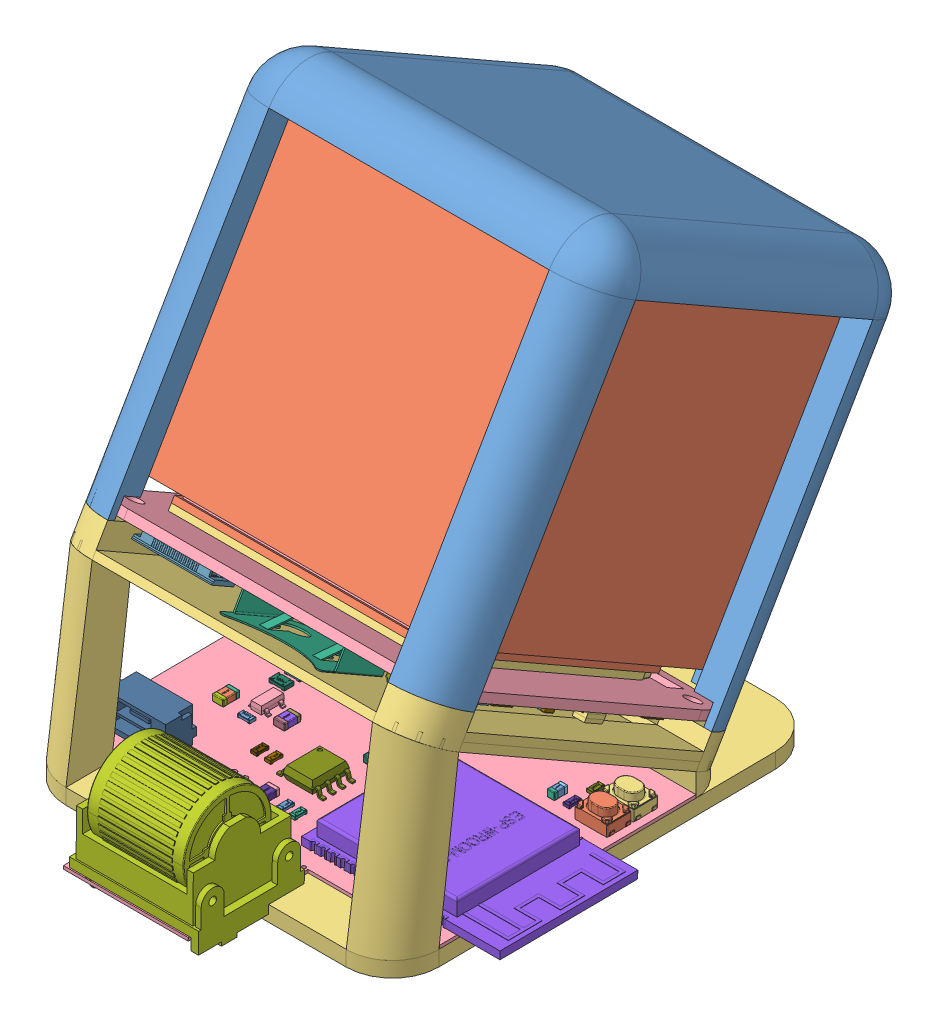
SolidWorks assembly main, configuration 默认. Lengths in mm.
Overall size (55.34 95.26 82.21).
436 component instances, 154 part files, 13 mates.
Components (placement in the parent):
- case-1: case [默认] at (0.5158 4.4817 0.3951) x (0.999924 -0.008726 -0.008727) z (0.01192 0.499915 0.865992) size (48 47.5 48)
- cubic-1: cubic [默认] at (0.3684 19.1653 -31.1742) x (0.999924 -0.008726 -0.008727) z (0.01192 0.499915 0.865992) size (40 40 40)
- stand-1: stand [默认] at (0.5158 4.4817 0.3951) x (0.01192 0.499915 0.865992) z (-0.999924 0.008726 0.008727) size (61.5 29.73 48.03)
- PCB_2020-12-27_16-28-50_2021-02-20_20-59-34-1: PCB_2020-12-27_16-28-50_2021-02-20_20-59-34 [默认] at (-66.8523 -25.1637 -60.1398) x (0.999924 -0.008726 -0.008727) z (-0.003194 -0.866031 0.499981) size (45.01 51.47 7.58)
  - PCB_2020-12-27_16-28-50_2021-02-20_20-59-34.step-1: PCB_2020-12-27_16-28-50_2021-02-20_20-59-34.step [默认] at origin size (45.01 51.47 7.58)
    - Board.step-1: Board.step [默认] at origin size (45.01 45.01 1.12)
      - Open CASCADE STEP translator 6.8 3.1.1.step-1: Open CASCADE STEP translator 6.8 3.1.1.step [默认] at (0 0 -1.1227) size (45.01 45.01 1.12)
    - C34.step-1: C34.step [默认] at origin size (2.2 1.45 0.88)
      - c0805c101k5gactu.step-1: c0805c101k5gactu.step [默认] at (159.963 120.323 -10.6426) x (1 0 0) z (0 -1 0) size (2.2 0.88 1.45)
        - Open CASCADE STEP translator 6.8 3.2.1.1.step-1: Open CASCADE STEP translator 6.8 3.2.1.1.step [默认] at origin size (2 0.86 1.43)
        - Open CASCADE STEP translator 6.8 3.2.1.2.step-1: Open CASCADE STEP translator 6.8 3.2.1.2.step [默认] at origin size (0.34 0 0.18)
        - Open CASCADE STEP translator 6.8 3.2.1.3.step-1: Open CASCADE STEP translator 6.8 3.2.1.3.step [默认] at origin size (0.41 0 0.18)
        - Open CASCADE STEP translator 6.8 3.2.1.4.step-1: Open CASCADE STEP translator 6.8 3.2.1.4.step [默认] at origin size (0.21 0 0.18)
        - Open CASCADE STEP translator 6.8 3.2.1.5.step-1: Open CASCADE STEP translator 6.8 3.2.1.5.step [默认] at origin size (0.5 0.88 1.45)
        - Open CASCADE STEP translator 6.8 3.2.1.6.step-1: Open CASCADE STEP translator 6.8 3.2.1.6.step [默认] at origin size (0.5 0.88 1.45)
    - C14.step-1: C14.step [默认] at origin size (1.45 2.2 0.88)
      - c0805c101k5gactu.step-1: c0805c101k5gactu.step [默认] at (101.7169 -30.907 -10.6426) x (0 -1 0) z (-1 0 0) size (2.2 0.88 1.45)
        - Open CASCADE STEP translator 6.8 3.2.1.1.step-1: Open CASCADE STEP translator 6.8 3.2.1.1.step [默认] at origin size (2 0.86 1.43)
        - Open CASCADE STEP translator 6.8 3.2.1.2.step-1: Open CASCADE STEP translator 6.8 3.2.1.2.step [默认] at origin size (0.34 0 0.18)
        - Open CASCADE STEP translator 6.8 3.2.1.3.step-1: Open CASCADE STEP translator 6.8 3.2.1.3.step [默认] at origin size (0.41 0 0.18)
        - Open CASCADE STEP translator 6.8 3.2.1.4.step-1: Open CASCADE STEP translator 6.8 3.2.1.4.step [默认] at origin size (0.21 0 0.18)
        - Open CASCADE STEP translator 6.8 3.2.1.5.step-1: Open CASCADE STEP translator 6.8 3.2.1.5.step [默认] at origin size (0.5 0.88 1.45)
        - Open CASCADE STEP translator 6.8 3.2.1.6.step-1: Open CASCADE STEP translator 6.8 3.2.1.6.step [默认] at origin size (0.5 0.88 1.45)
    - C13.step-1: C13.step [默认] at origin size (0.95 1.77 0.95)
      - c0603x104k3ractu.step-1: c0603x104k3ractu.step [默认] at (16.3625 164.212 -10.6426) x (0 1 0) z (1 0 0) size (1.77 0.95 0.95)
        - Open CASCADE STEP translator 6.8 3.4.1.1.step-1: Open CASCADE STEP translator 6.8 3.4.1.1.step [默认] at origin size (1.57 0.93 0.93)
        - Open CASCADE STEP translator 6.8 3.4.1.2.step-1: Open CASCADE STEP translator 6.8 3.4.1.2.step [默认] at origin size (0.24 0 0.13)
        - Open CASCADE STEP translator 6.8 3.4.1.3.step-1: Open CASCADE STEP translator 6.8 3.4.1.3.step [默认] at origin size (0.29 0 0.13)
        - Open CASCADE STEP translator 6.8 3.4.1.4.step-1: Open CASCADE STEP translator 6.8 3.4.1.4.step [默认] at origin size (0.15 0 0.13)
        - Open CASCADE STEP translator 6.8 3.4.1.5.step-1: Open CASCADE STEP translator 6.8 3.4.1.5.step [默认] at origin size (0.45 0.95 0.95)
        - Open CASCADE STEP translator 6.8 3.4.1.6.step-1: Open CASCADE STEP translator 6.8 3.4.1.6.step [默认] at origin size (0.45 0.95 0.95)
    - C12.step-1: C12.step [默认] at origin size (0.95 1.77 0.95)
      - c0603x104k3ractu.step-1: c0603x104k3ractu.step [默认] at (9.3976 164.422 -10.6426) x (0 1 0) z (1 0 0) size (1.77 0.95 0.95)
        - Open CASCADE STEP translator 6.8 3.4.1.1.step-1: Open CASCADE STEP translator 6.8 3.4.1.1.step [默认] at origin size (1.57 0.93 0.93)
        - Open CASCADE STEP translator 6.8 3.4.1.2.step-1: Open CASCADE STEP translator 6.8 3.4.1.2.step [默认] at origin size (0.24 0 0.13)
        - Open CASCADE STEP translator 6.8 3.4.1.3.step-1: Open CASCADE STEP translator 6.8 3.4.1.3.step [默认] at origin size (0.29 0 0.13)
        - Open CASCADE STEP translator 6.8 3.4.1.4.step-1: Open CASCADE STEP translator 6.8 3.4.1.4.step [默认] at origin size (0.15 0 0.13)
        - Open CASCADE STEP translator 6.8 3.4.1.5.step-1: Open CASCADE STEP translator 6.8 3.4.1.5.step [默认] at origin size (0.45 0.95 0.95)
        - Open CASCADE STEP translator 6.8 3.4.1.6.step-1: Open CASCADE STEP translator 6.8 3.4.1.6.step [默认] at origin size (0.45 0.95 0.95)
    - USB2.step-1: USB2.step [默认] at origin size (5 7.8 2.7)
      - User_Library-micro_usb_SMD_RGB8421504.step-1: User_Library-micro_usb_SMD_RGB8421504.step [默认] at (44.3599 67.8551 1.27) x (0 -1 0) z (-1 0 0) size (7.8 2.7 5)
    - R7.step-1: R7.step [默认] at origin size (1.6 0.8 0.42)
      - User_Library-Res-0603.step-1: User_Library-Res-0603.step [默认] at (87.122 80.8989 0) x (-1 0 0) z (0 1 0) size (1.6 0.42 0.8)
    - L2.step-1: L2.step [默认] at origin size (0.86 1.6 0.51)
      - CircuitWorks-RESISTOR_0603.step-1: CircuitWorks-RESISTOR_0603.step [默认] at (61.595 79.7559 0) x (0 -1 0) z (-1 0 0) size (1.6 0.51 0.86)
    - P2.step-1: P2.step [默认] at origin size (20.43 5.11 2.05)
      - 3-1734839-0_RGB8421504.step-1: 3-1734839-0_RGB8421504.step [默认] at (66.548 57.4041 1.0414) x (1 0 0) z (0 -1 0) size (20.43 2.05 5.11)
    - D4.step-1: D4.step [默认] at origin size (3.7 1.6 1.27)
      - CircuitWorks-SOD123.step-1: CircuitWorks-SOD123.step [默认] at (72.4968 69.5129 0.0508) x (1 0 0) z (0 -1 0) size (3.7 1.27 1.6)
    - D5.step-1: D5.step [默认] at origin size (1.6 3.7 1.27)
      - CircuitWorks-SOD123.step-1: CircuitWorks-SOD123.step [默认] at (87.6301 64.8969 0.0508) x (0 1 0) z (1 0 0) size (3.7 1.27 1.6)
    - C21.step-1: C21.step [默认] at origin size (1.45 2.2 0.88)
      - c0805c101k5gactu.step-1: c0805c101k5gactu.step [默认] at (98.5419 -33.828 -10.6426) x (0 -1 0) z (-1 0 0) size (2.2 0.88 1.45)
        - Open CASCADE STEP translator 6.8 3.2.1.1.step-1: Open CASCADE STEP translator 6.8 3.2.1.1.step [默认] at origin size (2 0.86 1.43)
        - Open CASCADE STEP translator 6.8 3.2.1.2.step-1: Open CASCADE STEP translator 6.8 3.2.1.2.step [默认] at origin size (0.34 0 0.18)
        - Open CASCADE STEP translator 6.8 3.2.1.3.step-1: Open CASCADE STEP translator 6.8 3.2.1.3.step [默认] at origin size (0.41 0 0.18)
        - Open CASCADE STEP translator 6.8 3.2.1.4.step-1: Open CASCADE STEP translator 6.8 3.2.1.4.step [默认] at origin size (0.21 0 0.18)
        - Open CASCADE STEP translator 6.8 3.2.1.5.step-1: Open CASCADE STEP translator 6.8 3.2.1.5.step [默认] at origin size (0.5 0.88 1.45)
        - Open CASCADE STEP translator 6.8 3.2.1.6.step-1: Open CASCADE STEP translator 6.8 3.2.1.6.step [默认] at origin size (0.5 0.88 1.45)
    - C24.step-1: C24.step [默认] at origin size (1.45 2.2 0.88)
      - c0805c101k5gactu.step-1: c0805c101k5gactu.step [默认] at (2.51 156.471 -10.6426) x (0 1 0) z (1 0 0) size (2.2 0.88 1.45)
        - Open CASCADE STEP translator 6.8 3.2.1.1.step-1: Open CASCADE STEP translator 6.8 3.2.1.1.step [默认] at origin size (2 0.86 1.43)
        - Open CASCADE STEP translator 6.8 3.2.1.2.step-1: Open CASCADE STEP translator 6.8 3.2.1.2.step [默认] at origin size (0.34 0 0.18)
        - Open CASCADE STEP translator 6.8 3.2.1.3.step-1: Open CASCADE STEP translator 6.8 3.2.1.3.step [默认] at origin size (0.41 0 0.18)
        - Open CASCADE STEP translator 6.8 3.2.1.4.step-1: Open CASCADE STEP translator 6.8 3.2.1.4.step [默认] at origin size (0.21 0 0.18)
        - Open CASCADE STEP translator 6.8 3.2.1.5.step-1: Open CASCADE STEP translator 6.8 3.2.1.5.step [默认] at origin size (0.5 0.88 1.45)
        - Open CASCADE STEP translator 6.8 3.2.1.6.step-1: Open CASCADE STEP translator 6.8 3.2.1.6.step [默认] at origin size (0.5 0.88 1.45)
    - U7.step-1: U7.step [默认] at origin size (2.5 3 1.1)
      - CircuitWorks-SOT-23-5.step-1: CircuitWorks-SOT-23-5.step [默认] at (84.308 68.2431 -0.5131) x (0 1 0) z (1 0 0) size (3 1.1 2.5)
    - U5.step-1: U5.step [默认] at origin size (7 7 0.55)
      - User_Library-UFQFPN48.step-1: User_Library-UFQFPN48.step [默认] at (57.0029 73.1959 0) x (-1 0 0) z (0 0 1) size (7 7 0.55)
    - R13.step-1: R13.step [默认] at origin size (0.8 1.6 0.42)
      - User_Library-Res-0603.step-1: User_Library-Res-0603.step [默认] at (78.3388 65.957 0) x (0 1 0) z (1 0 0) size (1.6 0.42 0.8)
    - U4.step-1: U4.step [默认] at origin size (19.57 12.72 3.54)
      - User_Library-BK-885-TR.step-1: User_Library-BK-885-TR.step [默认] at (69.4691 84.328 0) x (1 0 0) z (0 -1 0) size (19.57 3.54 12.72)
    - U3.step-1: U3.step [默认] at origin size (0.8 1.6 0.42)
      - User_Library-Res-0603.step-1: User_Library-Res-0603.step [默认] at (61.3211 52.876 0) x (0 -1 0) z (-1 0 0) size (1.6 0.42 0.8)
    - C27.step-1: C27.step [默认] at origin size (0.95 1.77 0.95)
      - c0603x104k3ractu.step-1: c0603x104k3ractu.step [默认] at (123.9324 -30.647 -10.6426) x (0 -1 0) z (-1 0 0) size (1.77 0.95 0.95)
        - Open CASCADE STEP translator 6.8 3.4.1.1.step-1: Open CASCADE STEP translator 6.8 3.4.1.1.step [默认] at origin size (1.57 0.93 0.93)
        - Open CASCADE STEP translator 6.8 3.4.1.2.step-1: Open CASCADE STEP translator 6.8 3.4.1.2.step [默认] at origin size (0.24 0 0.13)
        - Open CASCADE STEP translator 6.8 3.4.1.3.step-1: Open CASCADE STEP translator 6.8 3.4.1.3.step [默认] at origin size (0.29 0 0.13)
        - Open CASCADE STEP translator 6.8 3.4.1.4.step-1: Open CASCADE STEP translator 6.8 3.4.1.4.step [默认] at origin size (0.15 0 0.13)
        - Open CASCADE STEP translator 6.8 3.4.1.5.step-1: Open CASCADE STEP translator 6.8 3.4.1.5.step [默认] at origin size (0.45 0.95 0.95)
        - Open CASCADE STEP translator 6.8 3.4.1.6.step-1: Open CASCADE STEP translator 6.8 3.4.1.6.step [默认] at origin size (0.45 0.95 0.95)
    - C20.step-1: C20.step [默认] at origin size (3.7 1.95 1.8)
      - c1206x223j2gacauto.step-1: c1206x223j2gacauto.step [默认] at (174.9253 96.5054 -10.6426) x (1 0 0) z (0 -1 0) size (3.7 1.8 1.95)
        - Open CASCADE STEP translator 6.8 3.20.1.1.step-1: Open CASCADE STEP translator 6.8 3.20.1.1.step [默认] at origin size (3.5 1.78 1.93)
        - Open CASCADE STEP translator 6.8 3.20.1.2.step-1: Open CASCADE STEP translator 6.8 3.20.1.2.step [默认] at origin size (0.7 0 0.37)
        - Open CASCADE STEP translator 6.8 3.20.1.3.step-1: Open CASCADE STEP translator 6.8 3.20.1.3.step [默认] at origin size (0.85 0 0.37)
        - Open CASCADE STEP translator 6.8 3.20.1.4.step-1: Open CASCADE STEP translator 6.8 3.20.1.4.step [默认] at origin size (0.44 0 0.37)
        - Open CASCADE STEP translator 6.8 3.20.1.5.step-1: Open CASCADE STEP translator 6.8 3.20.1.5.step [默认] at origin size (0.6 1.8 1.95)
        - Open CASCADE STEP translator 6.8 3.20.1.6.step-1: Open CASCADE STEP translator 6.8 3.20.1.6.step [默认] at origin size (0.6 1.8 1.95)
    - X3.step-1: X3.step [默认] at origin size (1.5 3.2 0.91)
      - crystal_rtf3215.step-1: crystal_rtf3215.step [默认] at (66.167 69.4691 0) x (0 1 0) z (1 0 0) size (3.2 0.91 1.5)
    - C28.step-1: C28.step [默认] at origin size (1.45 2.2 0.88)
      - c0805c101k5gactu.step-1: c0805c101k5gactu.step [默认] at (25.644 150.077 -10.6426) x (0 1 0) z (1 0 0) size (2.2 0.88 1.45)
        - Open CASCADE STEP translator 6.8 3.2.1.1.step-1: Open CASCADE STEP translator 6.8 3.2.1.1.step [默认] at origin size (2 0.86 1.43)
        - Open CASCADE STEP translator 6.8 3.2.1.2.step-1: Open CASCADE STEP translator 6.8 3.2.1.2.step [默认] at origin size (0.34 0 0.18)
        - Open CASCADE STEP translator 6.8 3.2.1.3.step-1: Open CASCADE STEP translator 6.8 3.2.1.3.step [默认] at origin size (0.41 0 0.18)
        - Open CASCADE STEP translator 6.8 3.2.1.4.step-1: Open CASCADE STEP translator 6.8 3.2.1.4.step [默认] at origin size (0.21 0 0.18)
        - Open CASCADE STEP translator 6.8 3.2.1.5.step-1: Open CASCADE STEP translator 6.8 3.2.1.5.step [默认] at origin size (0.5 0.88 1.45)
        - Open CASCADE STEP translator 6.8 3.2.1.6.step-1: Open CASCADE STEP translator 6.8 3.2.1.6.step [默认] at origin size (0.5 0.88 1.45)
    - C29.step-1: C29.step [默认] at origin size (1.45 2.2 0.88)
      - c0805c101k5gactu.step-1: c0805c101k5gactu.step [默认] at (102.7329 -43.6071 -10.6426) x (0 -1 0) z (-1 0 0) size (2.2 0.88 1.45)
        - Open CASCADE STEP translator 6.8 3.2.1.1.step-1: Open CASCADE STEP translator 6.8 3.2.1.1.step [默认] at origin size (2 0.86 1.43)
        - Open CASCADE STEP translator 6.8 3.2.1.2.step-1: Open CASCADE STEP translator 6.8 3.2.1.2.step [默认] at origin size (0.34 0 0.18)
        - Open CASCADE STEP translator 6.8 3.2.1.3.step-1: Open CASCADE STEP translator 6.8 3.2.1.3.step [默认] at origin size (0.41 0 0.18)
        - Open CASCADE STEP translator 6.8 3.2.1.4.step-1: Open CASCADE STEP translator 6.8 3.2.1.4.step [默认] at origin size (0.21 0 0.18)
        - Open CASCADE STEP translator 6.8 3.2.1.5.step-1: Open CASCADE STEP translator 6.8 3.2.1.5.step [默认] at origin size (0.5 0.88 1.45)
        - Open CASCADE STEP translator 6.8 3.2.1.6.step-1: Open CASCADE STEP translator 6.8 3.2.1.6.step [默认] at origin size (0.5 0.88 1.45)
    - C30.step-1: C30.step [默认] at origin size (1.45 2.2 0.88)
      - c0805c101k5gactu.step-1: c0805c101k5gactu.step [默认] at (97.9069 -43.6071 -10.6426) x (0 -1 0) z (-1 0 0) size (2.2 0.88 1.45)
        - Open CASCADE STEP translator 6.8 3.2.1.1.step-1: Open CASCADE STEP translator 6.8 3.2.1.1.step [默认] at origin size (2 0.86 1.43)
        - Open CASCADE STEP translator 6.8 3.2.1.2.step-1: Open CASCADE STEP translator 6.8 3.2.1.2.step [默认] at origin size (0.34 0 0.18)
        - Open CASCADE STEP translator 6.8 3.2.1.3.step-1: Open CASCADE STEP translator 6.8 3.2.1.3.step [默认] at origin size (0.41 0 0.18)
        - Open CASCADE STEP translator 6.8 3.2.1.4.step-1: Open CASCADE STEP translator 6.8 3.2.1.4.step [默认] at origin size (0.21 0 0.18)
        - Open CASCADE STEP translator 6.8 3.2.1.5.step-1: Open CASCADE STEP translator 6.8 3.2.1.5.step [默认] at origin size (0.5 0.88 1.45)
        - Open CASCADE STEP translator 6.8 3.2.1.6.step-1: Open CASCADE STEP translator 6.8 3.2.1.6.step [默认] at origin size (0.5 0.88 1.45)
    - U6.step-1: U6.step [默认] at origin size (2.5 3 1.1)
      - CircuitWorks-SOT-23-5.step-1: CircuitWorks-SOT-23-5.step [默认] at (52.8119 59.0989 -0.5131) x (0 -1 0) z (-1 0 0) size (3 1.1 2.5)
    - FPC1.step-1: FPC1.step [默认] at origin size (12.1 6.6 2)
      - 52746-1290_RGB10066329.step-1: 52746-1290_RGB10066329.step [默认] at (53.7211 87.5031 0) x (1 0 0) z (0 -1 0) size (12.1 2 6.6)
    - C18.step-1: C18.step [默认] at origin size (0.95 1.77 0.95)
      - c0603x104k3ractu.step-1: c0603x104k3ractu.step [默认] at (29.9716 149.69 -10.6426) x (0 1 0) z (1 0 0) size (1.77 0.95 0.95)
        - Open CASCADE STEP translator 6.8 3.4.1.1.step-1: Open CASCADE STEP translator 6.8 3.4.1.1.step [默认] at origin size (1.57 0.93 0.93)
        - Open CASCADE STEP translator 6.8 3.4.1.2.step-1: Open CASCADE STEP translator 6.8 3.4.1.2.step [默认] at origin size (0.24 0 0.13)
        - Open CASCADE STEP translator 6.8 3.4.1.3.step-1: Open CASCADE STEP translator 6.8 3.4.1.3.step [默认] at origin size (0.29 0 0.13)
        - Open CASCADE STEP translator 6.8 3.4.1.4.step-1: Open CASCADE STEP translator 6.8 3.4.1.4.step [默认] at origin size (0.15 0 0.13)
        - Open CASCADE STEP translator 6.8 3.4.1.5.step-1: Open CASCADE STEP translator 6.8 3.4.1.5.step [默认] at origin size (0.45 0.95 0.95)
        - Open CASCADE STEP translator 6.8 3.4.1.6.step-1: Open CASCADE STEP translator 6.8 3.4.1.6.step [默认] at origin size (0.45 0.95 0.95)
    - X1.step-1: X1.step [默认] at origin size (2.5 3.2 1.05)
      - User_Library-SMD-3225_4P.step-1: User_Library-SMD-3225_4P.step [默认] at (70.338 73.8309 0) x (0 -1 0) z (0 0 1) size (3.2 2.5 1.05)
    - C26.step-1: C26.step [默认] at origin size (2.2 1.45 0.88)
      - c0805c101k5gactu.step-1: c0805c101k5gactu.step [默认] at (183.605 114.818 -10.6426) x (1 0 0) z (0 -1 0) size (2.2 0.88 1.45)
        - Open CASCADE STEP translator 6.8 3.2.1.1.step-1: Open CASCADE STEP translator 6.8 3.2.1.1.step [默认] at origin size (2 0.86 1.43)
        - Open CASCADE STEP translator 6.8 3.2.1.2.step-1: Open CASCADE STEP translator 6.8 3.2.1.2.step [默认] at origin size (0.34 0 0.18)
        - Open CASCADE STEP translator 6.8 3.2.1.3.step-1: Open CASCADE STEP translator 6.8 3.2.1.3.step [默认] at origin size (0.41 0 0.18)
        - Open CASCADE STEP translator 6.8 3.2.1.4.step-1: Open CASCADE STEP translator 6.8 3.2.1.4.step [默认] at origin size (0.21 0 0.18)
        - Open CASCADE STEP translator 6.8 3.2.1.5.step-1: Open CASCADE STEP translator 6.8 3.2.1.5.step [默认] at origin size (0.5 0.88 1.45)
        - Open CASCADE STEP translator 6.8 3.2.1.6.step-1: Open CASCADE STEP translator 6.8 3.2.1.6.step [默认] at origin size (0.5 0.88 1.45)
    - C25.step-1: C25.step [默认] at origin size (1.45 2.2 0.88)
      - c0805c101k5gactu.step-1: c0805c101k5gactu.step [默认] at (36.439 156.681 -10.6426) x (0 1 0) z (1 0 0) size (2.2 0.88 1.45)
        - Open CASCADE STEP translator 6.8 3.2.1.1.step-1: Open CASCADE STEP translator 6.8 3.2.1.1.step [默认] at origin size (2 0.86 1.43)
        - Open CASCADE STEP translator 6.8 3.2.1.2.step-1: Open CASCADE STEP translator 6.8 3.2.1.2.step [默认] at origin size (0.34 0 0.18)
        - Open CASCADE STEP translator 6.8 3.2.1.3.step-1: Open CASCADE STEP translator 6.8 3.2.1.3.step [默认] at origin size (0.41 0 0.18)
        - Open CASCADE STEP translator 6.8 3.2.1.4.step-1: Open CASCADE STEP translator 6.8 3.2.1.4.step [默认] at origin size (0.21 0 0.18)
        - Open CASCADE STEP translator 6.8 3.2.1.5.step-1: Open CASCADE STEP translator 6.8 3.2.1.5.step [默认] at origin size (0.5 0.88 1.45)
        - Open CASCADE STEP translator 6.8 3.2.1.6.step-1: Open CASCADE STEP translator 6.8 3.2.1.6.step [默认] at origin size (0.5 0.88 1.45)
    - R17.step-1: R17.step [默认] at origin size (1.6 0.8 0.42)
      - User_Library-Res-0603.step-1: User_Library-Res-0603.step [默认] at (65.278 55.7531 0) x (1 0 0) z (0 -1 0) size (1.6 0.42 0.8)
    - R12.step-1: R12.step [默认] at origin size (0.8 1.6 0.42)
      - User_Library-Res-0603.step-1: User_Library-Res-0603.step [默认] at (63.2461 52.832 0) x (0 -1 0) z (-1 0 0) size (1.6 0.42 0.8)
    - R16.step-1: R16.step [默认] at origin size (1.6 0.8 0.42)
      - User_Library-Res-0603.step-1: User_Library-Res-0603.step [默认] at (62.103 55.7529 0) x (-1 0 0) z (0 1 0) size (1.6 0.42 0.8)
    - R15.step-1: R15.step [默认] at origin size (0.8 1.6 0.42)
      - User_Library-Res-0603.step-1: User_Library-Res-0603.step [默认] at (65.0241 52.832 0) x (0 -1 0) z (-1 0 0) size (1.6 0.42 0.8)
    - SW2.step-1: SW2.step [默认] at origin size (4.6 3.2 2.5)
      - skrpace010_RGB10066329.step-1: skrpace010_RGB10066329.step [默认] at (82.5499 81.661 0) x (-1 0 0) z (0 1 0) size (4.6 2.5 3.2)
    - SW1.step-1: SW1.step [默认] at origin size (4.6 3.2 2.5)
      - skrpace010_RGB10066329.step-1: skrpace010_RGB10066329.step [默认] at (82.4231 85.217 0) x (1 0 0) z (0 -1 0) size (4.6 2.5 3.2)
    - C17.step-1: C17.step [默认] at origin size (1.77 0.95 0.95)
      - c0603x104k3ractu.step-1: c0603x104k3ractu.step [默认] at (159.977 114.6814 -10.6426) x (1 0 0) z (0 -1 0) size (1.77 0.95 0.95)
        - Open CASCADE STEP translator 6.8 3.4.1.1.step-1: Open CASCADE STEP translator 6.8 3.4.1.1.step [默认] at origin size (1.57 0.93 0.93)
        - Open CASCADE STEP translator 6.8 3.4.1.2.step-1: Open CASCADE STEP translator 6.8 3.4.1.2.step [默认] at origin size (0.24 0 0.13)
        - Open CASCADE STEP translator 6.8 3.4.1.3.step-1: Open CASCADE STEP translator 6.8 3.4.1.3.step [默认] at origin size (0.29 0 0.13)
        - Open CASCADE STEP translator 6.8 3.4.1.4.step-1: Open CASCADE STEP translator 6.8 3.4.1.4.step [默认] at origin size (0.15 0 0.13)
        - Open CASCADE STEP translator 6.8 3.4.1.5.step-1: Open CASCADE STEP translator 6.8 3.4.1.5.step [默认] at origin size (0.45 0.95 0.95)
        - Open CASCADE STEP translator 6.8 3.4.1.6.step-1: Open CASCADE STEP translator 6.8 3.4.1.6.step [默认] at origin size (0.45 0.95 0.95)
    - C19.step-1: C19.step [默认] at origin size (1.77 0.95 0.95)
      - c0603x104k3ractu.step-1: c0603x104k3ractu.step [默认] at (159.977 112.0144 -10.6426) x (1 0 0) z (0 -1 0) size (1.77 0.95 0.95)
        - Open CASCADE STEP translator 6.8 3.4.1.1.step-1: Open CASCADE STEP translator 6.8 3.4.1.1.step [默认] at origin size (1.57 0.93 0.93)
        - Open CASCADE STEP translator 6.8 3.4.1.2.step-1: Open CASCADE STEP translator 6.8 3.4.1.2.step [默认] at origin size (0.24 0 0.13)
        - Open CASCADE STEP translator 6.8 3.4.1.3.step-1: Open CASCADE STEP translator 6.8 3.4.1.3.step [默认] at origin size (0.29 0 0.13)
        - Open CASCADE STEP translator 6.8 3.4.1.4.step-1: Open CASCADE STEP translator 6.8 3.4.1.4.step [默认] at origin size (0.15 0 0.13)
        - Open CASCADE STEP translator 6.8 3.4.1.5.step-1: Open CASCADE STEP translator 6.8 3.4.1.5.step [默认] at origin size (0.45 0.95 0.95)
        - Open CASCADE STEP translator 6.8 3.4.1.6.step-1: Open CASCADE STEP translator 6.8 3.4.1.6.step [默认] at origin size (0.45 0.95 0.95)
    - C16.step-1: C16.step [默认] at origin size (1.77 0.95 0.95)
      - c0603x104k3ractu.step-1: c0603x104k3ractu.step [默认] at (163.64 118.7894 -10.6426) x (1 0 0) z (0 -1 0) size (1.77 0.95 0.95)
        - Open CASCADE STEP translator 6.8 3.4.1.1.step-1: Open CASCADE STEP translator 6.8 3.4.1.1.step [默认] at origin size (1.57 0.93 0.93)
        - Open CASCADE STEP translator 6.8 3.4.1.2.step-1: Open CASCADE STEP translator 6.8 3.4.1.2.step [默认] at origin size (0.24 0 0.13)
        - Open CASCADE STEP translator 6.8 3.4.1.3.step-1: Open CASCADE STEP translator 6.8 3.4.1.3.step [默认] at origin size (0.29 0 0.13)
        - Open CASCADE STEP translator 6.8 3.4.1.4.step-1: Open CASCADE STEP translator 6.8 3.4.1.4.step [默认] at origin size (0.15 0 0.13)
        - Open CASCADE STEP translator 6.8 3.4.1.5.step-1: Open CASCADE STEP translator 6.8 3.4.1.5.step [默认] at origin size (0.45 0.95 0.95)
        - Open CASCADE STEP translator 6.8 3.4.1.6.step-1: Open CASCADE STEP translator 6.8 3.4.1.6.step [默认] at origin size (0.45 0.95 0.95)
    - C15.step-1: C15.step [默认] at origin size (1.77 0.95 0.95)
      - c0603x104k3ractu.step-1: c0603x104k3ractu.step [默认] at (163.64 116.5034 -10.6426) x (1 0 0) z (0 -1 0) size (1.77 0.95 0.95)
        - Open CASCADE STEP translator 6.8 3.4.1.1.step-1: Open CASCADE STEP translator 6.8 3.4.1.1.step [默认] at origin size (1.57 0.93 0.93)
        - Open CASCADE STEP translator 6.8 3.4.1.2.step-1: Open CASCADE STEP translator 6.8 3.4.1.2.step [默认] at origin size (0.24 0 0.13)
        - Open CASCADE STEP translator 6.8 3.4.1.3.step-1: Open CASCADE STEP translator 6.8 3.4.1.3.step [默认] at origin size (0.29 0 0.13)
        - Open CASCADE STEP translator 6.8 3.4.1.4.step-1: Open CASCADE STEP translator 6.8 3.4.1.4.step [默认] at origin size (0.15 0 0.13)
        - Open CASCADE STEP translator 6.8 3.4.1.5.step-1: Open CASCADE STEP translator 6.8 3.4.1.5.step [默认] at origin size (0.45 0.95 0.95)
        - Open CASCADE STEP translator 6.8 3.4.1.6.step-1: Open CASCADE STEP translator 6.8 3.4.1.6.step [默认] at origin size (0.45 0.95 0.95)
    - R14.step-1: R14.step [默认] at origin size (0.8 1.6 0.42)
      - User_Library-Res-0603.step-1: User_Library-Res-0603.step [默认] at (76.4338 65.957 0) x (0 1 0) z (1 0 0) size (1.6 0.42 0.8)
    - R11.step-1: R11.step [默认] at origin size (3.2 2.51 0.55)
      - User_Library-RESC3225X06N.step-1: User_Library-RESC3225X06N.step [默认] at (72.4971 66.592 0) size (3.2 2.51 0.55)
    - C23.step-1: C23.step [默认] at origin size (1.45 2.2 0.88)
      - c0805c101k5gactu.step-1: c0805c101k5gactu.step [默认] at (92.0649 -37.257 -10.6426) x (0 -1 0) z (-1 0 0) size (2.2 0.88 1.45)
        - Open CASCADE STEP translator 6.8 3.2.1.1.step-1: Open CASCADE STEP translator 6.8 3.2.1.1.step [默认] at origin size (2 0.86 1.43)
        - Open CASCADE STEP translator 6.8 3.2.1.2.step-1: Open CASCADE STEP translator 6.8 3.2.1.2.step [默认] at origin size (0.34 0 0.18)
        - Open CASCADE STEP translator 6.8 3.2.1.3.step-1: Open CASCADE STEP translator 6.8 3.2.1.3.step [默认] at origin size (0.41 0 0.18)
        - Open CASCADE STEP translator 6.8 3.2.1.4.step-1: Open CASCADE STEP translator 6.8 3.2.1.4.step [默认] at origin size (0.21 0 0.18)
        - Open CASCADE STEP translator 6.8 3.2.1.5.step-1: Open CASCADE STEP translator 6.8 3.2.1.5.step [默认] at origin size (0.5 0.88 1.45)
        - Open CASCADE STEP translator 6.8 3.2.1.6.step-1: Open CASCADE STEP translator 6.8 3.2.1.6.step [默认] at origin size (0.5 0.88 1.45)
    - C22.step-1: C22.step [默认] at origin size (1.45 2.2 0.88)
      - c0805c101k5gactu.step-1: c0805c101k5gactu.step [默认] at (96.0019 -33.828 -10.6426) x (0 -1 0) z (-1 0 0) size (2.2 0.88 1.45)
        - Open CASCADE STEP translator 6.8 3.2.1.1.step-1: Open CASCADE STEP translator 6.8 3.2.1.1.step [默认] at origin size (2 0.86 1.43)
        - Open CASCADE STEP translator 6.8 3.2.1.2.step-1: Open CASCADE STEP translator 6.8 3.2.1.2.step [默认] at origin size (0.34 0 0.18)
        - Open CASCADE STEP translator 6.8 3.2.1.3.step-1: Open CASCADE STEP translator 6.8 3.2.1.3.step [默认] at origin size (0.41 0 0.18)
        - Open CASCADE STEP translator 6.8 3.2.1.4.step-1: Open CASCADE STEP translator 6.8 3.2.1.4.step [默认] at origin size (0.21 0 0.18)
        - Open CASCADE STEP translator 6.8 3.2.1.5.step-1: Open CASCADE STEP translator 6.8 3.2.1.5.step [默认] at origin size (0.5 0.88 1.45)
        - Open CASCADE STEP translator 6.8 3.2.1.6.step-1: Open CASCADE STEP translator 6.8 3.2.1.6.step [默认] at origin size (0.5 0.88 1.45)
    - LED2.step-1: LED2.step [默认] at origin size (3.6 3.5 0.95)
      - User_Library-WS2813_3535.step-1: User_Library-WS2813_3535.step [默认] at (47.732 54.273 0) x (1 0 0) z (0 -1 0) size (3.6 0.95 3.5)
    - LED3.step-1: LED3.step [默认] at origin size (3.6 3.5 0.95)
      - User_Library-WS2813_3535.step-1: User_Library-WS2813_3535.step [默认] at (47.732 77.133 0) x (1 0 0) z (0 -1 0) size (3.6 0.95 3.5)
    - LED5.step-1: LED5.step [默认] at origin size (3.6 3.5 0.95)
      - User_Library-WS2813_3535.step-1: User_Library-WS2813_3535.step [默认] at (85.324 54.273 0) x (1 0 0) z (0 -1 0) size (3.6 0.95 3.5)
    - LED4.step-1: LED4.step [默认] at origin size (3.6 3.5 0.95)
      - User_Library-WS2813_3535.step-1: User_Library-WS2813_3535.step [默认] at (85.324 77.133 0) x (1 0 0) z (0 -1 0) size (3.6 0.95 3.5)
    - C31.step-1: C31.step [默认] at origin size (1.45 2.2 0.88)
      - c0805c101k5gactu.step-1: c0805c101k5gactu.step [默认] at (115.199 -43.651 -10.6426) x (0 -1 0) z (-1 0 0) size (2.2 0.88 1.45)
        - Open CASCADE STEP translator 6.8 3.2.1.1.step-1: Open CASCADE STEP translator 6.8 3.2.1.1.step [默认] at origin size (2 0.86 1.43)
        - Open CASCADE STEP translator 6.8 3.2.1.2.step-1: Open CASCADE STEP translator 6.8 3.2.1.2.step [默认] at origin size (0.34 0 0.18)
        - Open CASCADE STEP translator 6.8 3.2.1.3.step-1: Open CASCADE STEP translator 6.8 3.2.1.3.step [默认] at origin size (0.41 0 0.18)
        - Open CASCADE STEP translator 6.8 3.2.1.4.step-1: Open CASCADE STEP translator 6.8 3.2.1.4.step [默认] at origin size (0.21 0 0.18)
        - Open CASCADE STEP translator 6.8 3.2.1.5.step-1: Open CASCADE STEP translator 6.8 3.2.1.5.step [默认] at origin size (0.5 0.88 1.45)
        - Open CASCADE STEP translator 6.8 3.2.1.6.step-1: Open CASCADE STEP translator 6.8 3.2.1.6.step [默认] at origin size (0.5 0.88 1.45)
    - C32.step-1: C32.step [默认] at origin size (1.45 2.2 0.88)
      - c0805c101k5gactu.step-1: c0805c101k5gactu.step [默认] at (13.178 150.121 -10.6426) x (0 1 0) z (1 0 0) size (2.2 0.88 1.45)
        - Open CASCADE STEP translator 6.8 3.2.1.1.step-1: Open CASCADE STEP translator 6.8 3.2.1.1.step [默认] at origin size (2 0.86 1.43)
        - Open CASCADE STEP translator 6.8 3.2.1.2.step-1: Open CASCADE STEP translator 6.8 3.2.1.2.step [默认] at origin size (0.34 0 0.18)
        - Open CASCADE STEP translator 6.8 3.2.1.3.step-1: Open CASCADE STEP translator 6.8 3.2.1.3.step [默认] at origin size (0.41 0 0.18)
        - Open CASCADE STEP translator 6.8 3.2.1.4.step-1: Open CASCADE STEP translator 6.8 3.2.1.4.step [默认] at origin size (0.21 0 0.18)
        - Open CASCADE STEP translator 6.8 3.2.1.5.step-1: Open CASCADE STEP translator 6.8 3.2.1.5.step [默认] at origin size (0.5 0.88 1.45)
        - Open CASCADE STEP translator 6.8 3.2.1.6.step-1: Open CASCADE STEP translator 6.8 3.2.1.6.step [默认] at origin size (0.5 0.88 1.45)
    - CN9.step-1: CN9.step [默认] at origin size (4.85 8.25 4.35)
      - User_Library-SM04B-GHS-TB_RGB14277081.step-1: User_Library-SM04B-GHS-TB_RGB14277081.step [默认] at (76.448 78.464 0) x (0 1 0) z (1 0 0) size (8.25 4.35 4.85)
    - C35.step-1: C35.step [默认] at origin size (1.77 0.95 0.95)
      - c0603x104k3ractu.step-1: c0603x104k3ractu.step [默认] at (-9.482 38.9886 -10.6426) x (-1 0 0) z (0 1 0) size (1.77 0.95 0.95)
        - Open CASCADE STEP translator 6.8 3.4.1.1.step-1: Open CASCADE STEP translator 6.8 3.4.1.1.step [默认] at origin size (1.57 0.93 0.93)
        - Open CASCADE STEP translator 6.8 3.4.1.2.step-1: Open CASCADE STEP translator 6.8 3.4.1.2.step [默认] at origin size (0.24 0 0.13)
        - Open CASCADE STEP translator 6.8 3.4.1.3.step-1: Open CASCADE STEP translator 6.8 3.4.1.3.step [默认] at origin size (0.29 0 0.13)
        - Open CASCADE STEP translator 6.8 3.4.1.4.step-1: Open CASCADE STEP translator 6.8 3.4.1.4.step [默认] at origin size (0.15 0 0.13)
        - Open CASCADE STEP translator 6.8 3.4.1.5.step-1: Open CASCADE STEP translator 6.8 3.4.1.5.step [默认] at origin size (0.45 0.95 0.95)
        - Open CASCADE STEP translator 6.8 3.4.1.6.step-1: Open CASCADE STEP translator 6.8 3.4.1.6.step [默认] at origin size (0.45 0.95 0.95)
    - C11.step-1: C11.step [默认] at origin size (1.77 0.95 0.95)
      - c0603x104k3ractu.step-1: c0603x104k3ractu.step [默认] at (149.436 121.6664 -10.6426) x (1 0 0) z (0 -1 0) size (1.77 0.95 0.95)
        - Open CASCADE STEP translator 6.8 3.4.1.1.step-1: Open CASCADE STEP translator 6.8 3.4.1.1.step [默认] at origin size (1.57 0.93 0.93)
        - Open CASCADE STEP translator 6.8 3.4.1.2.step-1: Open CASCADE STEP translator 6.8 3.4.1.2.step [默认] at origin size (0.24 0 0.13)
        - Open CASCADE STEP translator 6.8 3.4.1.3.step-1: Open CASCADE STEP translator 6.8 3.4.1.3.step [默认] at origin size (0.29 0 0.13)
        - Open CASCADE STEP translator 6.8 3.4.1.4.step-1: Open CASCADE STEP translator 6.8 3.4.1.4.step [默认] at origin size (0.15 0 0.13)
        - Open CASCADE STEP translator 6.8 3.4.1.5.step-1: Open CASCADE STEP translator 6.8 3.4.1.5.step [默认] at origin size (0.45 0.95 0.95)
        - Open CASCADE STEP translator 6.8 3.4.1.6.step-1: Open CASCADE STEP translator 6.8 3.4.1.6.step [默认] at origin size (0.45 0.95 0.95)
    - C36.step-1: C36.step [默认] at origin size (2.2 1.45 0.88)
      - c0805c101k5gactu.step-1: c0805c101k5gactu.step [默认] at (-43.651 36.312 -10.6426) x (-1 0 0) z (0 1 0) size (2.2 0.88 1.45)
        - Open CASCADE STEP translator 6.8 3.2.1.1.step-1: Open CASCADE STEP translator 6.8 3.2.1.1.step [默认] at origin size (2 0.86 1.43)
        - Open CASCADE STEP translator 6.8 3.2.1.2.step-1: Open CASCADE STEP translator 6.8 3.2.1.2.step [默认] at origin size (0.34 0 0.18)
        - Open CASCADE STEP translator 6.8 3.2.1.3.step-1: Open CASCADE STEP translator 6.8 3.2.1.3.step [默认] at origin size (0.41 0 0.18)
        - Open CASCADE STEP translator 6.8 3.2.1.4.step-1: Open CASCADE STEP translator 6.8 3.2.1.4.step [默认] at origin size (0.21 0 0.18)
        - Open CASCADE STEP translator 6.8 3.2.1.5.step-1: Open CASCADE STEP translator 6.8 3.2.1.5.step [默认] at origin size (0.5 0.88 1.45)
        - Open CASCADE STEP translator 6.8 3.2.1.6.step-1: Open CASCADE STEP translator 6.8 3.2.1.6.step [默认] at origin size (0.5 0.88 1.45)
    - C33.step-1: C33.step [默认] at origin size (1.77 0.95 0.95)
      - c0603x104k3ractu.step-1: c0603x104k3ractu.step [默认] at (-32.743 30.9046 -10.6426) x (-1 0 0) z (0 1 0) size (1.77 0.95 0.95)
        - Open CASCADE STEP translator 6.8 3.4.1.1.step-1: Open CASCADE STEP translator 6.8 3.4.1.1.step [默认] at origin size (1.57 0.93 0.93)
        - Open CASCADE STEP translator 6.8 3.4.1.2.step-1: Open CASCADE STEP translator 6.8 3.4.1.2.step [默认] at origin size (0.24 0 0.13)
        - Open CASCADE STEP translator 6.8 3.4.1.3.step-1: Open CASCADE STEP translator 6.8 3.4.1.3.step [默认] at origin size (0.29 0 0.13)
        - Open CASCADE STEP translator 6.8 3.4.1.4.step-1: Open CASCADE STEP translator 6.8 3.4.1.4.step [默认] at origin size (0.15 0 0.13)
        - Open CASCADE STEP translator 6.8 3.4.1.5.step-1: Open CASCADE STEP translator 6.8 3.4.1.5.step [默认] at origin size (0.45 0.95 0.95)
        - Open CASCADE STEP translator 6.8 3.4.1.6.step-1: Open CASCADE STEP translator 6.8 3.4.1.6.step [默认] at origin size (0.45 0.95 0.95)
    - Free-Models.step-1: Free-Models.step [默认] at origin size (33.8 46.35 1.8)
      - mcot128128az-rgbm.step-1: mcot128128az-rgbm.step [默认] at (83.7239 85.5761 -3.1293) x (-1 0 0) z (0 0 -1) size (33.8 46.35 1.8)
        - Open CASCADE STEP translator 6.8 3.56.1.1.step-1: Open CASCADE STEP translator 6.8 3.56.1.1.step [默认] at origin size (33.8 34 0.8)
        - Open CASCADE STEP translator 6.8 3.56.1.2.step-1: Open CASCADE STEP translator 6.8 3.56.1.2.step [默认] at origin size (33.8 32 0.8)
        - Open CASCADE STEP translator 6.8 3.56.1.3.step-1: Open CASCADE STEP translator 6.8 3.56.1.3.step [默认] at origin size (32.5 30.5 0.2)
        - Open CASCADE STEP translator 6.8 3.56.1.4.step-1: Open CASCADE STEP translator 6.8 3.56.1.4.step [默认] at origin size (28.86 28.86 0.1)
        - Open CASCADE STEP translator 6.8 3.56.1.5.step-1: Open CASCADE STEP translator 6.8 3.56.1.5.step [默认] at origin size (26.86 26.86 0.05)
        - Open CASCADE STEP translator 6.8 3.56.1.6.step-1: Open CASCADE STEP translator 6.8 3.56.1.6.step [默认] at origin size (27.83 14.35 0.12)
        - Open CASCADE STEP translator 6.8 3.56.1.7.step-1: Open CASCADE STEP translator 6.8 3.56.1.7.step [默认] at origin size (0.3 2 0.06)
        - Open CASCADE STEP translator 6.8 3.56.1.8.step-1: Open CASCADE STEP translator 6.8 3.56.1.8.step [默认] at origin size (0.3 2 0.06)
        - Open CASCADE STEP translator 6.8 3.56.1.9.step-1: Open CASCADE STEP translator 6.8 3.56.1.9.step [默认] at origin size (0.3 2 0.06)
        - Open CASCADE STEP translator 6.8 3.56.1.10.step-1: Open CASCADE STEP translator 6.8 3.56.1.10.step [默认] at origin size (0.3 2 0.06)
        - Open CASCADE STEP translator 6.8 3.56.1.11.step-1: Open CASCADE STEP translator 6.8 3.56.1.11.step [默认] at origin size (0.3 2 0.06)
        - Open CASCADE STEP translator 6.8 3.56.1.12.step-1: Open CASCADE STEP translator 6.8 3.56.1.12.step [默认] at origin size (0.3 2 0.06)
        - Open CASCADE STEP translator 6.8 3.56.1.13.step-1: Open CASCADE STEP translator 6.8 3.56.1.13.step [默认] at origin size (0.3 2 0.06)
        - Open CASCADE STEP translator 6.8 3.56.1.14.step-1: Open CASCADE STEP translator 6.8 3.56.1.14.step [默认] at origin size (0.3 2 0.06)
        - Open CASCADE STEP translator 6.8 3.56.1.15.step-1: Open CASCADE STEP translator 6.8 3.56.1.15.step [默认] at origin size (0.3 2 0.06)
        - Open CASCADE STEP translator 6.8 3.56.1.16.step-1: Open CASCADE STEP translator 6.8 3.56.1.16.step [默认] at origin size (0.3 2 0.06)
        - Open CASCADE STEP translator 6.8 3.56.1.17.step-1: Open CASCADE STEP translator 6.8 3.56.1.17.step [默认] at origin size (0.3 2 0.06)
        - Open CASCADE STEP translator 6.8 3.56.1.18.step-1: Open CASCADE STEP translator 6.8 3.56.1.18.step [默认] at origin size (0.3 2 0.06)
        - Open CASCADE STEP translator 6.8 3.56.1.19.step-1: Open CASCADE STEP translator 6.8 3.56.1.19.step [默认] at origin size (0.3 2 0.06)
        - Open CASCADE STEP translator 6.8 3.56.1.20.step-1: Open CASCADE STEP translator 6.8 3.56.1.20.step [默认] at origin size (0.3 2 0.06)
        - Open CASCADE STEP translator 6.8 3.56.1.21.step-1: Open CASCADE STEP translator 6.8 3.56.1.21.step [默认] at origin size (0.3 2 0.06)
        - Open CASCADE STEP translator 6.8 3.56.1.22.step-1: Open CASCADE STEP translator 6.8 3.56.1.22.step [默认] at origin size (0.3 2 0.06)
        - Open CASCADE STEP translator 6.8 3.56.1.23.step-1: Open CASCADE STEP translator 6.8 3.56.1.23.step [默认] at origin size (0.3 2 0.06)
        - Open CASCADE STEP translator 6.8 3.56.1.24.step-1: Open CASCADE STEP translator 6.8 3.56.1.24.step [默认] at origin size (0.3 2 0.06)
        - Open CASCADE STEP translator 6.8 3.56.1.25.step-1: Open CASCADE STEP translator 6.8 3.56.1.25.step [默认] at origin size (0.3 2 0.06)
        - Open CASCADE STEP translator 6.8 3.56.1.26.step-1: Open CASCADE STEP translator 6.8 3.56.1.26.step [默认] at origin size (0.3 2 0.06)
        - Open CASCADE STEP translator 6.8 3.56.1.27.step-1: Open CASCADE STEP translator 6.8 3.56.1.27.step [默认] at origin size (0.3 2 0.06)
        - Open CASCADE STEP translator 6.8 3.56.1.28.step-1: Open CASCADE STEP translator 6.8 3.56.1.28.step [默认] at origin size (0.3 2 0.06)
        - Open CASCADE STEP translator 6.8 3.56.1.29.step-1: Open CASCADE STEP translator 6.8 3.56.1.29.step [默认] at origin size (0.3 2 0.06)
        - Open CASCADE STEP translator 6.8 3.56.1.30.step-1: Open CASCADE STEP translator 6.8 3.56.1.30.step [默认] at origin size (0.3 2 0.06)
        - Open CASCADE STEP translator 6.8 3.56.1.31.step-1: Open CASCADE STEP translator 6.8 3.56.1.31.step [默认] at origin size (0.3 2 0.06)
        - Open CASCADE STEP translator 6.8 3.56.1.32.step-1: Open CASCADE STEP translator 6.8 3.56.1.32.step [默认] at origin size (0.3 2 0.06)
        - Open CASCADE STEP translator 6.8 3.56.1.33.step-1: Open CASCADE STEP translator 6.8 3.56.1.33.step [默认] at origin size (0.3 2 0.06)
        - Open CASCADE STEP translator 6.8 3.56.1.34.step-1: Open CASCADE STEP translator 6.8 3.56.1.34.step [默认] at origin size (0.3 2 0.06)
        - Open CASCADE STEP translator 6.8 3.56.1.35.step-1: Open CASCADE STEP translator 6.8 3.56.1.35.step [默认] at origin size (0.3 2 0.06)
        - Open CASCADE STEP translator 6.8 3.56.1.36.step-1: Open CASCADE STEP translator 6.8 3.56.1.36.step [默认] at origin size (0.3 2 0.06)
        - Open CASCADE STEP translator 6.8 3.56.1.37.step-1: Open CASCADE STEP translator 6.8 3.56.1.37.step [默认] at origin size (15.51 3 0.06)
        - Open CASCADE STEP translator 6.8 3.56.1.38.step-1: Open CASCADE STEP translator 6.8 3.56.1.38.step [默认] at origin size (33.8 2 0.8)
